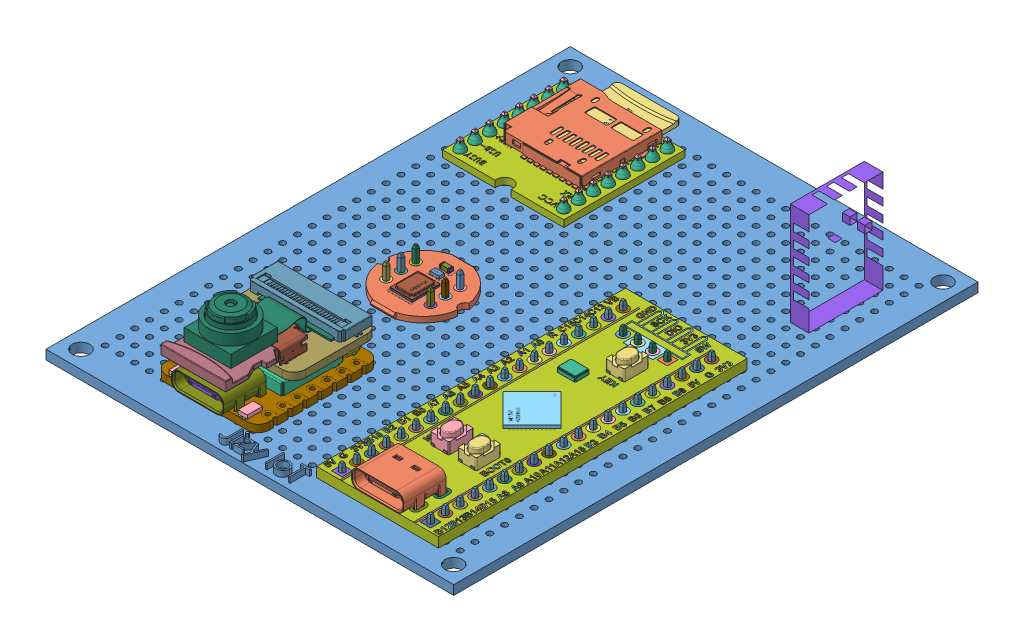
SolidWorks assembly 3D_Final, configuration Default. Lengths in mm.
Overall size (70 33.4 90).
323 component instances, 242 part files, 16 mates.
Components (placement in the parent):
- BoardDong7x9-1: BoardDong7x9 [Default] at (35 1.6 45) x (0 0 -1) z (0 1 0) size (90 70 2.6)
- blackpill v2.0 swi.STEP-1: blackpill v2.0 swi.STEP [Default] at (52.8 1.6 59.37) x (0 0 -1) z (0 1 0) size (53 20.9 10.45)
  - blackpill v2.0.step.STEP-1: blackpill v2.0.step.STEP [Default] at origin size (53 20.9 4.92)
    - USB Type C Port (SMD Type).step.STEP-1: USB Type C Port (SMD Type).step.STEP [Default] at (-19.2 0 3.305) x (0 -1 0) z (0 0 -1) size (8.94 7.9 4.2)
    - PTS810 SJK 250 SMTR LFS--3DModel-STEP-1.step.STEP-1: PTS810 SJK 250 SMTR LFS--3DModel-STEP-1.step.STEP [Default] at (14.5 -1.8498 1.7) x (1 0 0) z (0 -1 0) size (4.6 2.51 3.2)
    - PTS810 SJK 250 SMTR LFS--3DModel-STEP-1.step.STEP-2: PTS810 SJK 250 SMTR LFS--3DModel-STEP-1.step.STEP [Default] at (-11.4 -2.3498 1.7) x (1 0 0) z (0 -1 0) size (4.6 2.51 3.2)
    - PTS810 SJK 250 SMTR LFS--3DModel-STEP-1 v2(Mirror).step.STEP-1: PTS810 SJK 250 SMTR LFS--3DModel-STEP-1 v2(Mirror).step.STEP [Default] at (-11.4 2.3498 1.7) x (1 0 0) z (0 -1 0) size (4.6 2.51 3.2)
    - STM32F411CEU6.step.STEP-1: STM32F411CEU6.step.STEP [Default] at (0 0 1.7) x (-0.707107 -0.707107 0) z (-0.707107 0.707107 0) size (7 0.6 7)
    - ECS-135.60-12-33Q-JES-TR.step.STEP-1: ECS-135.60-12-33Q-JES-TR.step.STEP [Default] at (9.3867 2.3215 1.7) x (0 -1 0) z (-1 0 0) size (3.2 0.8 2.5)
    - DIY_black_pill.step.STEP-1: DIY_black_pill.step.STEP [Default] at origin size (53 20.9 1.7)
    - DIY_black_pill-0.step.STEP-1: DIY_black_pill-0.step.STEP [Default] at origin size (1.8 1.8 1.72)
    - DIY_black_pill-1.step.STEP-1: DIY_black_pill-1.step.STEP [Default] at origin size (1.8 1.8 1.72)
    - DIY_black_pill-2.step.STEP-1: DIY_black_pill-2.step.STEP [Default] at origin size (1.8 1.8 1.72)
    - DIY_black_pill-3.step.STEP-1: DIY_black_pill-3.step.STEP [Default] at origin size (1.8 1.8 1.72)
    - DIY_black_pill-4.step.STEP-1: DIY_black_pill-4.step.STEP [Default] at origin size (1.8 1.8 1.72)
    - DIY_black_pill-5.step.STEP-1: DIY_black_pill-5.step.STEP [Default] at origin size (1.8 1.8 1.72)
    - DIY_black_pill-6.step.STEP-1: DIY_black_pill-6.step.STEP [Default] at origin size (1.8 1.8 1.72)
    - DIY_black_pill-7.step.STEP-1: DIY_black_pill-7.step.STEP [Default] at origin size (1.8 1.8 1.72)
    - DIY_black_pill-8.step.STEP-1: DIY_black_pill-8.step.STEP [Default] at origin size (1.8 1.8 1.72)
    - DIY_black_pill-9.step.STEP-1: DIY_black_pill-9.step.STEP [Default] at origin size (1.8 1.8 1.72)
    - DIY_black_pill-10.step.STEP-1: DIY_black_pill-10.step.STEP [Default] at origin size (1.8 1.8 1.72)
    - DIY_black_pill-11.step.STEP-1: DIY_black_pill-11.step.STEP [Default] at origin size (1.8 1.8 1.72)
    - DIY_black_pill-12.step.STEP-1: DIY_black_pill-12.step.STEP [Default] at origin size (1.8 1.8 1.72)
    - DIY_black_pill-13.step.STEP-1: DIY_black_pill-13.step.STEP [Default] at origin size (1.8 1.8 1.72)
    - DIY_black_pill-14.step.STEP-1: DIY_black_pill-14.step.STEP [Default] at origin size (1.8 1.8 1.72)
    - DIY_black_pill-15.step.STEP-1: DIY_black_pill-15.step.STEP [Default] at origin size (1.8 1.8 1.72)
    - DIY_black_pill-16.step.STEP-1: DIY_black_pill-16.step.STEP [Default] at origin size (1.8 1.8 1.72)
    - DIY_black_pill-17.step.STEP-1: DIY_black_pill-17.step.STEP [Default] at origin size (1.8 1.8 1.72)
    - DIY_black_pill-18.step.STEP-1: DIY_black_pill-18.step.STEP [Default] at origin size (1.8 1.8 1.72)
    - DIY_black_pill-19.step.STEP-1: DIY_black_pill-19.step.STEP [Default] at origin size (1.8 1.8 1.72)
    - DIY_black_pill-20.step.STEP-1: DIY_black_pill-20.step.STEP [Default] at origin size (1.8 1.8 1.72)
    - DIY_black_pill-21.step.STEP-1: DIY_black_pill-21.step.STEP [Default] at origin size (1.8 1.8 1.72)
    - DIY_black_pill-22.step.STEP-1: DIY_black_pill-22.step.STEP [Default] at origin size (1.8 1.8 1.72)
    - DIY_black_pill-23.step.STEP-1: DIY_black_pill-23.step.STEP [Default] at origin size (1.8 1.8 1.72)
    - DIY_black_pill-24.step.STEP-1: DIY_black_pill-24.step.STEP [Default] at origin size (1.8 1.8 1.72)
    - DIY_black_pill-25.step.STEP-1: DIY_black_pill-25.step.STEP [Default] at origin size (1.8 1.8 1.72)
    - DIY_black_pill-26.step.STEP-1: DIY_black_pill-26.step.STEP [Default] at origin size (1.8 1.8 1.72)
    - DIY_black_pill-27.step.STEP-1: DIY_black_pill-27.step.STEP [Default] at origin size (1.8 1.8 1.72)
    - DIY_black_pill-28.step.STEP-1: DIY_black_pill-28.step.STEP [Default] at origin size (1.8 1.8 1.72)
    - DIY_black_pill-29.step.STEP-1: DIY_black_pill-29.step.STEP [Default] at origin size (1.8 1.8 1.72)
    - DIY_black_pill-30.step.STEP-1: DIY_black_pill-30.step.STEP [Default] at origin size (1.8 1.8 1.72)
    - DIY_black_pill-31.step.STEP-1: DIY_black_pill-31.step.STEP [Default] at origin size (1.8 1.8 1.72)
    - DIY_black_pill-32.step.STEP-1: DIY_black_pill-32.step.STEP [Default] at origin size (1.8 1.8 1.72)
    - DIY_black_pill-33.step.STEP-1: DIY_black_pill-33.step.STEP [Default] at origin size (1.8 1.8 1.72)
    - DIY_black_pill-34.step.STEP-1: DIY_black_pill-34.step.STEP [Default] at origin size (1.8 1.8 1.72)
    - DIY_black_pill-35.step.STEP-1: DIY_black_pill-35.step.STEP [Default] at origin size (1.8 1.8 1.72)
    - DIY_black_pill-36.step.STEP-1: DIY_black_pill-36.step.STEP [Default] at origin size (1.8 1.8 1.72)
    - DIY_black_pill-37.step.STEP-1: DIY_black_pill-37.step.STEP [Default] at origin size (1.8 1.8 1.72)
    - DIY_black_pill-38.step.STEP-1: DIY_black_pill-38.step.STEP [Default] at origin size (1.8 1.8 1.72)
    - DIY_black_pill-39.step.STEP-1: DIY_black_pill-39.step.STEP [Default] at origin size (1.8 1.8 1.72)
    - DIY_black_pill-40.step.STEP-1: DIY_black_pill-40.step.STEP [Default] at origin size (51.2 0.3 0.01)
    - DIY_black_pill-41.step.STEP-1: DIY_black_pill-41.step.STEP [Default] at origin size (51.2 0.3 0.01)
    - DIY_black_pill-42.step.STEP-1: DIY_black_pill-42.step.STEP [Default] at origin size (0.93 1 0.01)
    - DIY_black_pill-43.step.STEP-1: DIY_black_pill-43.step.STEP [Default] at origin size (0.94 1.03 0.01)
    - DIY_black_pill-44.step.STEP-1: DIY_black_pill-44.step.STEP [Default] at origin size (0.93 1 0.01)
    - DIY_black_pill-45.step.STEP-1: DIY_black_pill-45.step.STEP [Default] at origin size (0.67 1.02 0.01)
    - DIY_black_pill-46.step.STEP-1: DIY_black_pill-46.step.STEP [Default] at origin size (0.66 1.02 0.01)
    - DIY_black_pill-47.step.STEP-1: DIY_black_pill-47.step.STEP [Default] at origin size (0.84 1 0.01)
    - DIY_black_pill-48.step.STEP-1: DIY_black_pill-48.step.STEP [Default] at origin size (0.67 1.02 0.01)
    - DIY_black_pill-49.step.STEP-1: DIY_black_pill-49.step.STEP [Default] at origin size (0.84 1.01 0.01)
    - DIY_black_pill-50.step.STEP-1: DIY_black_pill-50.step.STEP [Default] at origin size (0.72 1.01 0.01)
    - DIY_black_pill-51.step.STEP-1: DIY_black_pill-51.step.STEP [Default] at origin size (0.84 1 0.01)
    - DIY_black_pill-52.step.STEP-1: DIY_black_pill-52.step.STEP [Default] at origin size (0.67 1 0.01)
    - DIY_black_pill-53.step.STEP-1: DIY_black_pill-53.step.STEP [Default] at origin size (1 1 0.01)
    - DIY_black_pill-54.step.STEP-1: DIY_black_pill-54.step.STEP [Default] at origin size (0.44 1 0.01)
    - DIY_black_pill-55.step.STEP-1: DIY_black_pill-55.step.STEP [Default] at origin size (0.44 1 0.01)
    - DIY_black_pill-56.step.STEP-1: DIY_black_pill-56.step.STEP [Default] at origin size (1 1 0.01)
    - DIY_black_pill-57.step.STEP-1: DIY_black_pill-57.step.STEP [Default] at origin size (0.44 1 0.01)
    - DIY_black_pill-58.step.STEP-1: DIY_black_pill-58.step.STEP [Default] at origin size (0.67 1.02 0.01)
    - DIY_black_pill-59.step.STEP-1: DIY_black_pill-59.step.STEP [Default] at origin size (0.66 1.02 0.01)
    - DIY_black_pill-60.step.STEP-1: DIY_black_pill-60.step.STEP [Default] at origin size (0.67 1 0.01)
    - DIY_black_pill-61.step.STEP-1: DIY_black_pill-61.step.STEP [Default] at origin size (0.84 1 0.01)
    - DIY_black_pill-62.step.STEP-1: DIY_black_pill-62.step.STEP [Default] at origin size (0.44 1 0.01)
    - DIY_black_pill-63.step.STEP-1: DIY_black_pill-63.step.STEP [Default] at origin size (0.66 1.02 0.01)
    - DIY_black_pill-64.step.STEP-1: DIY_black_pill-64.step.STEP [Default] at origin size (0.44 1 0.01)
    - DIY_black_pill-65.step.STEP-1: DIY_black_pill-65.step.STEP [Default] at origin size (0.84 1 0.01)
    - DIY_black_pill-66.step.STEP-1: DIY_black_pill-66.step.STEP [Default] at origin size (0.72 1 0.01)
    - DIY_black_pill-67.step.STEP-1: DIY_black_pill-67.step.STEP [Default] at origin size (0.44 1 0.01)
    - DIY_black_pill-68.step.STEP-1: DIY_black_pill-68.step.STEP [Default] at origin size (0.84 1 0.01)
    - DIY_black_pill-69.step.STEP-1: DIY_black_pill-69.step.STEP [Default] at origin size (1 1 0.01)
    - DIY_black_pill-70.step.STEP-1: DIY_black_pill-70.step.STEP [Default] at origin size (1 1 0.01)
    - DIY_black_pill-71.step.STEP-1: DIY_black_pill-71.step.STEP [Default] at origin size (0.65 1.02 0.01)
    - DIY_black_pill-72.step.STEP-1: DIY_black_pill-72.step.STEP [Default] at origin size (0.44 1 0.01)
    - DIY_black_pill-73.step.STEP-1: DIY_black_pill-73.step.STEP [Default] at origin size (1 1 0.01)
    - DIY_black_pill-74.step.STEP-1: DIY_black_pill-74.step.STEP [Default] at origin size (0.67 1 0.01)
    - DIY_black_pill-75.step.STEP-1: DIY_black_pill-75.step.STEP [Default] at origin size (0.44 1 0.01)
    - DIY_black_pill-76.step.STEP-1: DIY_black_pill-76.step.STEP [Default] at origin size (1 1 0.01)
    - DIY_black_pill-77.step.STEP-1: DIY_black_pill-77.step.STEP [Default] at origin size (0.66 1.02 0.01)
    - DIY_black_pill-78.step.STEP-1: DIY_black_pill-78.step.STEP [Default] at origin size (0.84 1.01 0.01)
    - DIY_black_pill-79.step.STEP-1: DIY_black_pill-79.step.STEP [Default] at origin size (0.67 1.01 0.01)
    - DIY_black_pill-80.step.STEP-1: DIY_black_pill-80.step.STEP [Default] at origin size (0.84 1 0.01)
    - DIY_black_pill-81.step.STEP-1: DIY_black_pill-81.step.STEP [Default] at origin size (0.66 0.99 0.01)
    - DIY_black_pill-82.step.STEP-1: DIY_black_pill-82.step.STEP [Default] at origin size (0.84 1 0.01)
    - DIY_black_pill-83.step.STEP-1: DIY_black_pill-83.step.STEP [Default] at origin size (0.84 1 0.01)
    - DIY_black_pill-84.step.STEP-1: DIY_black_pill-84.step.STEP [Default] at origin size (0.67 1 0.01)
    - DIY_black_pill-85.step.STEP-1: DIY_black_pill-85.step.STEP [Default] at origin size (0.66 1.02 0.01)
    - DIY_black_pill-86.step.STEP-1: DIY_black_pill-86.step.STEP [Default] at origin size (0.66 1.02 0.01)
    - DIY_black_pill-87.step.STEP-1: DIY_black_pill-87.step.STEP [Default] at origin size (0.67 1 0.01)
    - DIY_black_pill-88.step.STEP-1: DIY_black_pill-88.step.STEP [Default] at origin size (0.44 1 0.01)
    - DIY_black_pill-89.step.STEP-1: DIY_black_pill-89.step.STEP [Default] at origin size (0.84 1 0.01)
    - DIY_black_pill-90.step.STEP-1: DIY_black_pill-90.step.STEP [Default] at origin size (1 1 0.01)
    - DIY_black_pill-91.step.STEP-1: DIY_black_pill-91.step.STEP [Default] at origin size (0.84 1 0.01)
    - DIY_black_pill-92.step.STEP-1: DIY_black_pill-92.step.STEP [Default] at origin size (0.44 1 0.01)
    - DIY_black_pill-93.step.STEP-1: DIY_black_pill-93.step.STEP [Default] at origin size (0.87 1.03 0.01)
    - DIY_black_pill-94.step.STEP-1: DIY_black_pill-94.step.STEP [Default] at origin size (0.44 1 0.01)
    - DIY_black_pill-95.step.STEP-1: DIY_black_pill-95.step.STEP [Default] at origin size (0.44 1 0.01)
    - DIY_black_pill-96.step.STEP-1: DIY_black_pill-96.step.STEP [Default] at origin size (0.9 1 0.01)
    - DIY_black_pill-97.step.STEP-1: DIY_black_pill-97.step.STEP [Default] at origin size (0.65 1.02 0.01)
    - DIY_black_pill-98.step.STEP-1: DIY_black_pill-98.step.STEP [Default] at origin size (1 1 0.01)
    - DIY_black_pill-99.step.STEP-1: DIY_black_pill-99.step.STEP [Default] at origin size (0.72 1 0.01)
    - DIY_black_pill-100.step.STEP-1: DIY_black_pill-100.step.STEP [Default] at origin size (1 1 0.01)
    - DIY_black_pill-101.step.STEP-1: DIY_black_pill-101.step.STEP [Default] at origin size (0.67 1.02 0.01)
    - DIY_black_pill-102.step.STEP-1: DIY_black_pill-102.step.STEP [Default] at origin size (0.65 1.02 0.01)
    - DIY_black_pill-103.step.STEP-1: DIY_black_pill-103.step.STEP [Default] at origin size (1 1 0.01)
    - DIY_black_pill-104.step.STEP-1: DIY_black_pill-104.step.STEP [Default] at origin size (0.84 1 0.01)
    - DIY_black_pill-105.step.STEP-1: DIY_black_pill-105.step.STEP [Default] at origin size (0.84 1 0.01)
    - DIY_black_pill-106.step.STEP-1: DIY_black_pill-106.step.STEP [Default] at origin size (0.65 1.02 0.01)
    - DIY_black_pill-107.step.STEP-1: DIY_black_pill-107.step.STEP [Default] at origin size (0.66 1.02 0.01)
    - DIY_black_pill-108.step.STEP-1: DIY_black_pill-108.step.STEP [Default] at origin size (0.66 1.02 0.01)
    - DIY_black_pill-109.step.STEP-1: DIY_black_pill-109.step.STEP [Default] at origin size (0.67 1 0.01)
    - DIY_black_pill-110.step.STEP-1: DIY_black_pill-110.step.STEP [Default] at origin size (0.93 1 0.01)
    - DIY_black_pill-111.step.STEP-1: DIY_black_pill-111.step.STEP [Default] at origin size (0.94 1.03 0.01)
    - DIY_black_pill-112.step.STEP-1: DIY_black_pill-112.step.STEP [Default] at origin size (0.93 1 0.01)
    - DIY_black_pill-113.step.STEP-1: DIY_black_pill-113.step.STEP [Default] at origin size (0.44 1 0.01)
    - DIY_black_pill-114.step.STEP-1: DIY_black_pill-114.step.STEP [Default] at origin size (0.84 1 0.01)
    - DIY_black_pill-115.step.STEP-1: DIY_black_pill-115.step.STEP [Default] at origin size (0.67 1 0.01)
    - DIY_black_pill-116.step.STEP-1: DIY_black_pill-116.step.STEP [Default] at origin size (0.44 1 0.01)
    - DIY_black_pill-117.step.STEP-1: DIY_black_pill-117.step.STEP [Default] at origin size (0.66 0.99 0.01)
    - DIY_black_pill-118.step.STEP-1: DIY_black_pill-118.step.STEP [Default] at origin size (0.84 1 0.01)
    - DIY_black_pill-119.step.STEP-1: DIY_black_pill-119.step.STEP [Default] at origin size (1 1 0.01)
    - DIY_black_pill-120.step.STEP-1: DIY_black_pill-120.step.STEP [Default] at origin size (0.67 1 0.01)
    - DIY_black_pill-121.step.STEP-1: DIY_black_pill-121.step.STEP [Default] at origin size (1 1 0.01)
    - DIY_black_pill-122.step.STEP-1: DIY_black_pill-122.step.STEP [Default] at origin size (0.66 1.02 0.01)
    - DIY_black_pill-123.step.STEP-1: DIY_black_pill-123.step.STEP [Default] at origin size (1 1 0.01)
    - DIY_black_pill-124.step.STEP-1: DIY_black_pill-124.step.STEP [Default] at origin size (0.67 1 0.01)
    - DIY_black_pill-125.step.STEP-1: DIY_black_pill-125.step.STEP [Default] at origin size (0.87 1.03 0.01)
    - DIY_black_pill-126.step.STEP-1: DIY_black_pill-126.step.STEP [Default] at origin size (0.72 1 0.01)
    - DIY_black_pill-127.step.STEP-1: DIY_black_pill-127.step.STEP [Default] at origin size (0.66 1.02 0.01)
    - DIY_black_pill-128.step.STEP-1: DIY_black_pill-128.step.STEP [Default] at origin size (0.87 1.03 0.01)
    - DIY_black_pill-129.step.STEP-1: DIY_black_pill-129.step.STEP [Default] at origin size (0.93 1 0.01)
    - DIY_black_pill-130.step.STEP-1: DIY_black_pill-130.step.STEP [Default] at origin size (0.44 1 0.01)
    - DIY_black_pill-131.step.STEP-1: DIY_black_pill-131.step.STEP [Default] at origin size (2.55 1.5 1.72)
    - DIY_black_pill-132.step.STEP-1: DIY_black_pill-132.step.STEP [Default] at origin size (2.6 1.5 1.72)
    - DIY_black_pill-133.step.STEP-1: DIY_black_pill-133.step.STEP [Default] at origin size (2.55 1.5 1.72)
    - DIY_black_pill-134.step.STEP-1: DIY_black_pill-134.step.STEP [Default] at origin size (2.6 1.5 1.72)
    - DIY_black_pill-135.step.STEP-1: DIY_black_pill-135.step.STEP [Default] at origin size (1 1 0.01)
    - DIY_black_pill-136.step.STEP-1: DIY_black_pill-136.step.STEP [Default] at origin size (0.67 1.01 0.01)
    - DIY_black_pill-137.step.STEP-1: DIY_black_pill-137.step.STEP [Default] at origin size (1.8 1.8 1.72)
    - DIY_black_pill-138.step.STEP-1: DIY_black_pill-138.step.STEP [Default] at origin size (1.8 1.8 1.72)
    - DIY_black_pill-139.step.STEP-1: DIY_black_pill-139.step.STEP [Default] at origin size (1.8 1.8 1.72)
    - DIY_black_pill-140.step.STEP-1: DIY_black_pill-140.step.STEP [Default] at origin size (1.8 1.8 1.72)
    - DIY_black_pill-141.step.STEP-1: DIY_black_pill-141.step.STEP [Default] at origin size (8.17 10.16 0.01)
    - DIY_black_pill-142.step.STEP-1: DIY_black_pill-142.step.STEP [Default] at origin size (1.31 1 0.01)
    - DIY_black_pill-143.step.STEP-1: DIY_black_pill-143.step.STEP [Default] at origin size (0.93 1 0.01)
    - DIY_black_pill-144.step.STEP-1: DIY_black_pill-144.step.STEP [Default] at origin size (0.84 1 0.01)
    - DIY_black_pill-145.step.STEP-1: DIY_black_pill-145.step.STEP [Default] at origin size (0.2 1 0.01)
    - DIY_black_pill-146.step.STEP-1: DIY_black_pill-146.step.STEP [Default] at origin size (0.87 1.03 0.01)
    - DIY_black_pill-147.step.STEP-1: DIY_black_pill-147.step.STEP [Default] at origin size (0.94 1.03 0.01)
    - DIY_black_pill-148.step.STEP-1: DIY_black_pill-148.step.STEP [Default] at origin size (0.79 1 0.01)
    - DIY_black_pill-149.step.STEP-1: DIY_black_pill-149.step.STEP [Default] at origin size (0.84 1 0.01)
    - DIY_black_pill-150.step.STEP-1: DIY_black_pill-150.step.STEP [Default] at origin size (0.9 1 0.01)
    - DIY_black_pill-151.step.STEP-1: DIY_black_pill-151.step.STEP [Default] at origin size (0.81 1.03 0.01)
    - DIY_black_pill-152.step.STEP-1: DIY_black_pill-152.step.STEP [Default] at origin size (0.97 1.03 0.01)
    - DIY_black_pill-153.step.STEP-1: DIY_black_pill-153.step.STEP [Default] at origin size (0.66 1.02 0.01)
    - DIY_black_pill-154.step.STEP-1: DIY_black_pill-154.step.STEP [Default] at origin size (0.66 1.02 0.01)
    - DIY_black_pill-155.step.STEP-1: DIY_black_pill-155.step.STEP [Default] at origin size (0.81 1.03 0.01)
    - DIY_black_pill-156.step.STEP-1: DIY_black_pill-156.step.STEP [Default] at origin size (0.9 1 0.01)
    - DIY_black_pill-157.step.STEP-1: DIY_black_pill-157.step.STEP [Default] at origin size (0.81 1.03 0.01)
    - DIY_black_pill-158.step.STEP-1: DIY_black_pill-158.step.STEP [Default] at origin size (0.97 1.03 0.01)
    - DIY_black_pill-159.step.STEP-1: DIY_black_pill-159.step.STEP [Default] at origin size (0.97 1.03 0.01)
    - DIY_black_pill-160.step.STEP-1: DIY_black_pill-160.step.STEP [Default] at origin size (1.01 0.91 0.01)
    - DIY_black_pill-161.step.STEP-1: DIY_black_pill-161.step.STEP [Default] at origin size (1 0.94 0.01)
    - DIY_black_pill-162.step.STEP-1: DIY_black_pill-162.step.STEP [Default] at origin size (1 0.77 0.01)
    - DIY_black_pill-163.step.STEP-1: DIY_black_pill-163.step.STEP [Default] at origin size (0.79 1 0.01)
    - DIY_black_pill-164.step.STEP-1: DIY_black_pill-164.step.STEP [Default] at origin size (0.65 1.02 0.01)
    - DIY_black_pill-165.step.STEP-1: DIY_black_pill-165.step.STEP [Default] at origin size (0.84 1 0.01)
    - DIY_black_pill-166.step.STEP-1: DIY_black_pill-166.step.STEP [Default] at origin size (0.79 1 0.01)
    - DIY_black_pill-167.step.STEP-1: DIY_black_pill-167.step.STEP [Default] at origin size (0.79 1 0.01)
  - 1x20 Male Pin Header.STEP-1: 1x20 Male Pin Header.STEP [Default] at (23.26 -7.6 0) x (-1 0 0) z (0 -1 0) size (50.8 8.54 2.5)
  - 1x20 Male Pin Header.STEP-2: 1x20 Male Pin Header.STEP [Default] at (23.26 7.6 0) x (-1 0 0) z (0 -1 0) size (50.8 8.54 2.5)
  - 1x4 Male Pin Header.STEP-1: 1x4 Male Pin Header.STEP [Default] at (19.45 -3.81 0) x (0 1 0) z (-1 0 0) size (10.17 8.54 2.5)
- Seeed Studio XIAO-ESP32-S3-Sense-1: Seeed Studio XIAO-ESP32-S3-Sense [Default] at (16.1886 1.85 72.4693) x (0 0 1) z (-1 0 0) size (24.36 13.98 17.79)
  - Seeed Studio XIAO-ESP32-S3-Sense.step-1: Seeed Studio XIAO-ESP32-S3-Sense.step [Default] at origin size (24.36 13.98 17.79)
    - Seeed Studio XIAO-ESP32-S3 (Sense).step-1: Seeed Studio XIAO-ESP32-S3 (Sense).step [Default] at origin size (22.49 4.48 17.79)
      - USB TYPE C PORT.step-1: USB TYPE C PORT.step [Default] at (4.3161 13.395 -12.1571) x (0 0 -1) z (0 -1 0) size (8.94 7.9 4.2)
        - USB TYPE C PORT (1).step-1: USB TYPE C PORT (1).step [Default] at (-3.0192 1.0963 5.395) size (8.94 7.9 4.2)
          - BOSS-EXTRUDE14_8_.step-1: BOSS-EXTRUDE14_8_.step [Default] at (-3.0192 1.0963 5.395) size (0.6 1 0.3)
          - BOSS-EXTRUDE7_4_.step-1: BOSS-EXTRUDE7_4_.step [Default] at (-3.0192 1.0963 5.395) size (0.3 3.78 0.75)
          - BOSS-EXTRUDE7_3_.step-1: BOSS-EXTRUDE7_3_.step [Default] at (-3.0192 1.0963 5.395) size (0.3 3.78 0.75)
          - BOSS-EXTRUDE14_4_.step-1: BOSS-EXTRUDE14_4_.step [Default] at (-3.0192 1.0963 5.395) size (0.3 1 0.3)
          - BOSS-EXTRUDE14_2_.step-1: BOSS-EXTRUDE14_2_.step [Default] at (-3.0192 1.0963 5.395) size (0.6 1 0.3)
          - BOSS-EXTRUDE14_11_.step-1: BOSS-EXTRUDE14_11_.step [Default] at (-3.0192 1.0963 5.395) size (0.3 1 0.3)
          - BOSS-EXTRUDE7_7_.step-1: BOSS-EXTRUDE7_7_.step [Default] at (-3.0192 1.0963 5.395) size (0.3 3.78 0.75)
          - BOSS-EXTRUDE14_9_.step-1: BOSS-EXTRUDE14_9_.step [Default] at (-3.0192 1.0963 5.395) size (0.3 1 0.3)
          - BOSS-EXTRUDE14_3_.step-1: BOSS-EXTRUDE14_3_.step [Default] at (-3.0192 1.0963 5.395) size (0.3 1 0.3)
          - BOSS-EXTRUDE14_7_.step-1: BOSS-EXTRUDE14_7_.step [Default] at (-3.0192 1.0963 5.395) size (0.6 1 0.3)
          - MIRROR2.step-1: MIRROR2.step [Default] at (-3.0192 1.0963 5.395) size (6.7 4.6 0.7)
          - BOSS-EXTRUDE14_5_.step-1: BOSS-EXTRUDE14_5_.step [Default] at (-3.0192 1.0963 5.395) size (0.3 1 0.3)
          - BOSS-EXTRUDE14_12_.step-1: BOSS-EXTRUDE14_12_.step [Default] at (-3.0192 1.0963 5.395) size (0.3 1 0.3)
          - BOSS-EXTRUDE7_8_.step-1: BOSS-EXTRUDE7_8_.step [Default] at (-3.0192 1.0963 5.395) size (0.3 3.78 0.75)
          - BOSS-EXTRUDE7_1_.step-1: BOSS-EXTRUDE7_1_.step [Default] at (-3.0192 1.0963 5.395) size (0.3 3.78 0.75)
          - BOSS-EXTRUDE14_10_.step-1: BOSS-EXTRUDE14_10_.step [Default] at (-3.0192 1.0963 5.395) size (0.3 1 0.3)
          - BOSS-EXTRUDE7_9_.step-1: BOSS-EXTRUDE7_9_.step [Default] at (-3.0192 1.0963 5.395) size (0.3 3.78 0.75)
          - BOSS-EXTRUDE14_6_.step-1: BOSS-EXTRUDE14_6_.step [Default] at (-3.0192 1.0963 5.395) size (0.6 1 0.3)
          - CHAMFER9.step-1: CHAMFER9.step [Default] at (-3.0192 1.0963 5.395) size (8.94 7.3 4.2)
          - BOSS-EXTRUDE14_1_.step-1: BOSS-EXTRUDE14_1_.step [Default] at (-3.0192 1.0963 5.395) size (0.3 1 0.3)
          - BOSS-EXTRUDE7_6_.step-1: BOSS-EXTRUDE7_6_.step [Default] at (-3.0192 1.0963 5.395) size (0.3 3.78 0.75)
          - BOSS-EXTRUDE7_2_.step-1: BOSS-EXTRUDE7_2_.step [Default] at (-3.0192 1.0963 5.395) size (0.3 3.78 0.75)
          - CUT-EXTRUDE5.step-1: CUT-EXTRUDE5.step [Default] at (-3.0192 1.0963 5.395) size (8.54 2 3.59)
          - BOSS-EXTRUDE7_5_.step-1: BOSS-EXTRUDE7_5_.step [Default] at (-3.0192 1.0963 5.395) size (0.3 3.78 0.75)
      - SKTAAAE010 v1.step-1: SKTAAAE010 v1.step [Default] at (10.7092 1 -12.0449) x (1 0 0) z (0 1 0) size (3.09 1.6 0.73)
        - Body.step-1: Body.step [Default] at (0 0 0.1) size (2.6 1.6 0.63)
        - Pins.step-1: Pins.step [Default] at origin size (3.09 1.19 0.1)
      - SKTAAAE010 v1.step-2: SKTAAAE010 v1.step [Default] at (10.6911 1 -0.1868) x (1 0 0) z (0 1 0) size (3.09 1.6 0.73)
        - Body.step-1: Body.step [Default] at (0 0 0.1) size (2.6 1.6 0.63)
        - Pins.step-1: Pins.step [Default] at origin size (3.09 1.19 0.1)
      - Shield.step-1: Shield.step [Default] at origin size (10.6 2.7 12.6)
      - U.FL-R-SMT-1_10_ v1.step-1: U.FL-R-SMT-1_10_ v1.step [Default] at (-6.9517 1 -10.8381) x (1 0 0) z (0 1 0) size (3 3.1 1.25)
      - DF40C-30DP-0.4V_51_ v1.step-1: DF40C-30DP-0.4V_51_ v1.step [Default] at (-6.0667 1.65 -7.7227) size (2.97 1.14 7.52)
      - Seeed Studio XIAO-ESP32-S3 (Sense)-0.step-1: Seeed Studio XIAO-ESP32-S3 (Sense)-0.step [Default] at origin size (20.97 1.28 17.79)
    - Sense Expansion Board.step-1: Sense Expansion Board.step [Default] at (-0.3 4.5 0) x (-1 0 0) z (0 0 1) size (24.36 7.23 16.78)
      - DF40HC(3.0)-30DS.step-1: DF40HC(3.0)-30DS.step [Default] at (6.4217 1.57 -3.0777) x (-1 0 0) z (0 0 1) size (3.38 2.9 8.6)
      - 10067099-200LF v1.step-1: 10067099-200LF v1.step [Default] at (-1.3077 -2.08 -6.0846) x (0 0 -1) z (-1 0 0) size (11.4 2.65 5.5)
      - PCB.step-1: PCB.step [Default] at origin size (14.68 1.25 16.78)
      - MicroSD v2.step-1: MicroSD v2.step [Default] at (-8.16 -2.1 -6.9267) x (1 0 0) z (0 0 -1) size (15.06 1.66 11.19)
      - JUSHUO AFC01-S24FCA-00.step-1: JUSHUO AFC01-S24FCA-00.step [Default] at (6.9932 -0.67 -6.0797) x (0 0 1) z (0 -1 0) size (16.2 6.01 2.01)
    - Camer Module.step-1: Camer Module.step [Default] at (-7.2 6 -13) size (19.95 8.11 12.5)
- INMP441 I2S Microphone Module v15-1: INMP441 I2S Microphone Module v15 [Default] at (23.57 1.6 48.81) size (13.77 11.25 14.24)
  - INMP441 I2S Microphone Module v15.step-1: INMP441 I2S Microphone Module v15.step [Default] at origin size (13.77 11.25 14.24)
    - C0603_070.step-1: C0603_070.step [Default] at (0 8.5 0) x (1 0 0) z (0 1 0) size (1.6 0.8 0.7)
      - C0603_070_1.step-1: C0603_070_1.step [Default] at origin size (1.6 0.8 0.7)
        - Part 3.step-1: Part 3.step [Default] at (0 4 -7.535) size (1.4 0.77 0.67)
        - Part 2.step-1: Part 2.step [Default] at (0 4 -7.535) size (0.2 0.8 0.7)
        - Part 1.step-1: Part 1.step [Default] at (0 4 -7.535) size (0.2 0.8 0.7)
    - 0603 Resistor.step-1: 0603 Resistor.step [Default] at (0 0.98 -2.4) x (1 0 0) z (0 1 0) size (1.6 0.9 0.5)
    - INMP441 I2S Microphone Module.step-1: INMP441 I2S Microphone Module.step [Default] at origin size (13.77 1 14.24)
    - INMP441 I2S Microphone Module-0.step-1: INMP441 I2S Microphone Module-0.step [Default] at origin size (1.6 1 1.6)
    - INMP441 I2S Microphone Module-1.step-1: INMP441 I2S Microphone Module-1.step [Default] at origin size (1.6 1 1.6)
    - INMP441 I2S Microphone Module-2.step-1: INMP441 I2S Microphone Module-2.step [Default] at origin size (1.6 1 1.6)
    - INMP441 I2S Microphone Module-3.step-1: INMP441 I2S Microphone Module-3.step [Default] at origin size (1.6 1 1.6)
    - INMP441 I2S Microphone Module-4.step-1: INMP441 I2S Microphone Module-4.step [Default] at origin size (1.6 1 1.6)
    - INMP441 I2S Microphone Module-5.step-1: INMP441 I2S Microphone Module-5.step [Default] at origin size (1.6 1 1.6)
    - INMP441 I2S Microphone Module-6.step-1: INMP441 I2S Microphone Module-6.step [Default] at origin size (1.6 1 1.6)
    - INMP441 I2S Microphone Module-7.step-1: INMP441 I2S Microphone Module-7.step [Default] at origin size (3.79 0.3 4.79)
    - INMP441 I2S Microphone Module-8.step-1: INMP441 I2S Microphone Module-8.step [Default] at origin size (3.79 0.41 4.79)
    - INMP441 I2S Microphone Module-9.step-1: INMP441 I2S Microphone Module-9.step [Default] at origin size (0.65 11.25 0.65)
    - INMP441 I2S Microphone Module-10.step-1: INMP441 I2S Microphone Module-10.step [Default] at origin size (2.55 2.5 7.63)
    - INMP441 I2S Microphone Module-11.step-1: INMP441 I2S Microphone Module-11.step [Default] at origin size (0.65 11.25 0.65)
    - INMP441 I2S Microphone Module-12.step-1: INMP441 I2S Microphone Module-12.step [Default] at origin size (0.65 11.25 0.65)
    - INMP441 I2S Microphone Module-13.step-1: INMP441 I2S Microphone Module-13.step [Default] at origin size (0.65 11.25 0.65)
    - INMP441 I2S Microphone Module-14.step-1: INMP441 I2S Microphone Module-14.step [Default] at origin size (2.55 2.5 7.63)
    - INMP441 I2S Microphone Module-15.step-1: INMP441 I2S Microphone Module-15.step [Default] at origin size (0.65 11.25 0.65)
    - INMP441 I2S Microphone Module-16.step-1: INMP441 I2S Microphone Module-16.step [Default] at origin size (0.65 11.25 0.65)
- DFPlayer Mini Assem v1.step-1: DFPlayer Mini Assem v1.step [Default] at (15.95 1.6 17.06) x (-1 0 0) z (0 0 -1) size (20.8 11.2 23.46)
  - SD card Assem^DFPlayer Mini Assem v1.step-1: SD card Assem^DFPlayer Mini Assem v1.step [Default] at (-198.0203 122.5536 -43.8714) x (0 1 0) z (1 0 0) size (2.44 17.9 16) (virtual)
    - CD card slot^SD card Assem_DFPlayer Mini Assem v1.step-1: CD card slot^SD card Assem_DFPlayer Mini Assem v1.step [Default] at (-120.5536 47.0914 197.6703) x (0 0 1) z (1 0 0) size (16 15 2.44) (virtual)
    - Micro sd card^SD card Assem_DFPlayer Mini Assem v1.step-1: Micro sd card^SD card Assem_DFPlayer Mini Assem v1.step [Default] at (-120.5536 45.5089 151.9853) x (0 0 1) z (1 0 0) size (11 15 0.95) (virtual)
  - DFPlayer Mini Pin.step-1: DFPlayer Mini Pin.step [Default] at (8.89 0 8.89) x (0 0 -1) z (0 -1 0) size (2.54 2.54 11.2)
    - 11_20mm pin.step-1: 11_20mm pin.step [Default] at (0 0 2.6) size (0.63 0.63 11.2)
    - Pin Header 1x12 TH Pitch 2.step-1: Pin Header 1x12 TH Pitch 2.step [Default] at (-27.94 0 -0.0014) size (2.54 2.54 2.8)
    - solder.step-1: solder.step [Default] at (0 0 -1.15) x (1 0 0) z (0 1 0) size (1.8 1.45 1.8)
  - DFPlayer Mini Pin.step-2: DFPlayer Mini Pin.step [Default] at (-8.89 0 8.89) x (0 0 1) z (0 -1 0) size (2.54 2.54 11.2)
    - 11_20mm pin.step-1: 11_20mm pin.step [Default] at (0 0 2.6) size (0.63 0.63 11.2)
    - Pin Header 1x12 TH Pitch 2.step-1: Pin Header 1x12 TH Pitch 2.step [Default] at (-27.94 0 -0.0014) size (2.54 2.54 2.8)
    - solder.step-1: solder.step [Default] at (0 0 -1.15) x (1 0 0) z (0 1 0) size (1.8 1.45 1.8)
  - DFPlayer Mini Pin.step-3: DFPlayer Mini Pin.step [Default] at (-8.89 0 6.35) x (0 0 1) z (0 -1 0) size (2.54 2.54 11.2)
    - 11_20mm pin.step-1: 11_20mm pin.step [Default] at (0 0 2.6) size (0.63 0.63 11.2)
    - Pin Header 1x12 TH Pitch 2.step-1: Pin Header 1x12 TH Pitch 2.step [Default] at (-27.94 0 -0.0014) size (2.54 2.54 2.8)
    - solder.step-1: solder.step [Default] at (0 0 -1.15) x (1 0 0) z (0 1 0) size (1.8 1.45 1.8)
  - DFPlayer Mini Pin.step-4: DFPlayer Mini Pin.step [Default] at (-8.89 0 3.81) x (0 0 1) z (0 -1 0) size (2.54 2.54 11.2)
    - 11_20mm pin.step-1: 11_20mm pin.step [Default] at (0 0 2.6) size (0.63 0.63 11.2)
    - Pin Header 1x12 TH Pitch 2.step-1: Pin Header 1x12 TH Pitch 2.step [Default] at (-27.94 0 -0.0014) size (2.54 2.54 2.8)
    - solder.step-1: solder.step [Default] at (0 0 -1.15) x (1 0 0) z (0 1 0) size (1.8 1.45 1.8)
  - DFPlayer Mini Pin.step-5: DFPlayer Mini Pin.step [Default] at (-8.89 0 1.27) x (0 0 1) z (0 -1 0) size (2.54 2.54 11.2)
    - 11_20mm pin.step-1: 11_20mm pin.step [Default] at (0 0 2.6) size (0.63 0.63 11.2)
    - Pin Header 1x12 TH Pitch 2.step-1: Pin Header 1x12 TH Pitch 2.step [Default] at (-27.94 0 -0.0014) size (2.54 2.54 2.8)
    - solder.step-1: solder.step [Default] at (0 0 -1.15) x (1 0 0) z (0 1 0) size (1.8 1.45 1.8)
  - DFPlayer Mini Pin.step-6: DFPlayer Mini Pin.step [Default] at (-8.89 0 -1.27) x (0 0 1) z (0 -1 0) size (2.54 2.54 11.2)
    - 11_20mm pin.step-1: 11_20mm pin.step [Default] at (0 0 2.6) size (0.63 0.63 11.2)
    - Pin Header 1x12 TH Pitch 2.step-1: Pin Header 1x12 TH Pitch 2.step [Default] at (-27.94 0 -0.0014) size (2.54 2.54 2.8)
    - solder.step-1: solder.step [Default] at (0 0 -1.15) x (1 0 0) z (0 1 0) size (1.8 1.45 1.8)
  - DFPlayer Mini Pin.step-7: DFPlayer Mini Pin.step [Default] at (-8.89 0 -3.81) x (0 0 1) z (0 -1 0) size (2.54 2.54 11.2)
    - 11_20mm pin.step-1: 11_20mm pin.step [Default] at (0 0 2.6) size (0.63 0.63 11.2)
    - Pin Header 1x12 TH Pitch 2.step-1: Pin Header 1x12 TH Pitch 2.step [Default] at (-27.94 0 -0.0014) size (2.54 2.54 2.8)
    - solder.step-1: solder.step [Default] at (0 0 -1.15) x (1 0 0) z (0 1 0) size (1.8 1.45 1.8)
  - DFPlayer Mini Pin.step-8: DFPlayer Mini Pin.step [Default] at (-8.89 0 -6.35) x (0 0 1) z (0 -1 0) size (2.54 2.54 11.2)
    - 11_20mm pin.step-1: 11_20mm pin.step [Default] at (0 0 2.6) size (0.63 0.63 11.2)
    - Pin Header 1x12 TH Pitch 2.step-1: Pin Header 1x12 TH Pitch 2.step [Default] at (-27.94 0 -0.0014) size (2.54 2.54 2.8)
    - solder.step-1: solder.step [Default] at (0 0 -1.15) x (1 0 0) z (0 1 0) size (1.8 1.45 1.8)
  - DFPlayer Mini Pin.step-9: DFPlayer Mini Pin.step [Default] at (-8.89 0 -8.89) x (0 0 1) z (0 -1 0) size (2.54 2.54 11.2)
    - 11_20mm pin.step-1: 11_20mm pin.step [Default] at (0 0 2.6) size (0.63 0.63 11.2)
    - Pin Header 1x12 TH Pitch 2.step-1: Pin Header 1x12 TH Pitch 2.step [Default] at (-27.94 0 -0.0014) size (2.54 2.54 2.8)
    - solder.step-1: solder.step [Default] at (0 0 -1.15) x (1 0 0) z (0 1 0) size (1.8 1.45 1.8)
  - DFPlayer Mini Pin.step-10: DFPlayer Mini Pin.step [Default] at (8.89 0 6.35) x (0 0 -1) z (0 -1 0) size (2.54 2.54 11.2)
    - 11_20mm pin.step-1: 11_20mm pin.step [Default] at (0 0 2.6) size (0.63 0.63 11.2)
    - Pin Header 1x12 TH Pitch 2.step-1: Pin Header 1x12 TH Pitch 2.step [Default] at (-27.94 0 -0.0014) size (2.54 2.54 2.8)
    - solder.step-1: solder.step [Default] at (0 0 -1.15) x (1 0 0) z (0 1 0) size (1.8 1.45 1.8)
  - DFPlayer Mini Pin.step-11: DFPlayer Mini Pin.step [Default] at (8.89 0 3.81) x (0 0 -1) z (0 -1 0) size (2.54 2.54 11.2)
    - 11_20mm pin.step-1: 11_20mm pin.step [Default] at (0 0 2.6) size (0.63 0.63 11.2)
    - Pin Header 1x12 TH Pitch 2.step-1: Pin Header 1x12 TH Pitch 2.step [Default] at (-27.94 0 -0.0014) size (2.54 2.54 2.8)
    - solder.step-1: solder.step [Default] at (0 0 -1.15) x (1 0 0) z (0 1 0) size (1.8 1.45 1.8)
  - DFPlayer Mini Pin.step-12: DFPlayer Mini Pin.step [Default] at (8.89 0 1.27) x (0 0 -1) z (0 -1 0) size (2.54 2.54 11.2)
    - 11_20mm pin.step-1: 11_20mm pin.step [Default] at (0 0 2.6) size (0.63 0.63 11.2)
    - Pin Header 1x12 TH Pitch 2.step-1: Pin Header 1x12 TH Pitch 2.step [Default] at (-27.94 0 -0.0014) size (2.54 2.54 2.8)
    - solder.step-1: solder.step [Default] at (0 0 -1.15) x (1 0 0) z (0 1 0) size (1.8 1.45 1.8)
  - DFPlayer Mini Pin.step-13: DFPlayer Mini Pin.step [Default] at (8.89 0 -1.27) x (0 0 -1) z (0 -1 0) size (2.54 2.54 11.2)
    - 11_20mm pin.step-1: 11_20mm pin.step [Default] at (0 0 2.6) size (0.63 0.63 11.2)
    - Pin Header 1x12 TH Pitch 2.step-1: Pin Header 1x12 TH Pitch 2.step [Default] at (-27.94 0 -0.0014) size (2.54 2.54 2.8)
    - solder.step-1: solder.step [Default] at (0 0 -1.15) x (1 0 0) z (0 1 0) size (1.8 1.45 1.8)
  - DFPlayer Mini Pin.step-14: DFPlayer Mini Pin.step [Default] at (8.89 0 -3.81) x (0 0 -1) z (0 -1 0) size (2.54 2.54 11.2)
    - 11_20mm pin.step-1: 11_20mm pin.step [Default] at (0 0 2.6) size (0.63 0.63 11.2)
    - Pin Header 1x12 TH Pitch 2.step-1: Pin Header 1x12 TH Pitch 2.step [Default] at (-27.94 0 -0.0014) size (2.54 2.54 2.8)
    - solder.step-1: solder.step [Default] at (0 0 -1.15) x (1 0 0) z (0 1 0) size (1.8 1.45 1.8)
  - DFPlayer Mini Pin.step-15: DFPlayer Mini Pin.step [Default] at (8.89 0 -6.35) x (0 0 -1) z (0 -1 0) size (2.54 2.54 11.2)
    - 11_20mm pin.step-1: 11_20mm pin.step [Default] at (0 0 2.6) size (0.63 0.63 11.2)
    - Pin Header 1x12 TH Pitch 2.step-1: Pin Header 1x12 TH Pitch 2.step [Default] at (-27.94 0 -0.0014) size (2.54 2.54 2.8)
    - solder.step-1: solder.step [Default] at (0 0 -1.15) x (1 0 0) z (0 1 0) size (1.8 1.45 1.8)
  - DFPlayer Mini Pin.step-16: DFPlayer Mini Pin.step [Default] at (8.89 0 -8.89) x (0 0 -1) z (0 -1 0) size (2.54 2.54 11.2)
    - 11_20mm pin.step-1: 11_20mm pin.step [Default] at (0 0 2.6) size (0.63 0.63 11.2)
    - Pin Header 1x12 TH Pitch 2.step-1: Pin Header 1x12 TH Pitch 2.step [Default] at (-27.94 0 -0.0014) size (2.54 2.54 2.8)
    - solder.step-1: solder.step [Default] at (0 0 -1.15) x (1 0 0) z (0 1 0) size (1.8 1.45 1.8)
  - DFPlayer Mini PCB^DFPlayer Mini Assem v1.step-1: DFPlayer Mini PCB^DFPlayer Mini Assem v1.step [Default] at origin size (20.8 1.15 20.8) (virtual)
- DHT22-1: DHT22 [Default] at (60.4 1.6 20.87) x (0 0 -1) z (0 1 0) size (15.33 7.8 27.74)
Mates (geometry in assembly coordinates):
- Concentric1: concentric aligned: cylinder of BoardDong7x9-1 through (60.4 0 84.37) axis (0 1 0) radius 0.5; circle of blackpill v2.0 swi.STEP-1/blackpill v2.0.step.STEP-1/DIY_black_pill-20.step.STEP-1
- Parallel1: parallel aligned: plane of BoardDong7x9-1 through (70 0 0) normal (1 0 0); plane of blackpill v2.0 swi.STEP-1/blackpill v2.0.step.STEP-1/DIY_black_pill.step.STEP-1 through (63.25 1.6 85.87) normal (1 0 0)
- Coincident2: coincident anti-aligned: plane of BoardDong7x9-1 through (35 1.6 45) normal (0 1 0); plane of blackpill v2.0 swi.STEP-1/blackpill v2.0.step.STEP-1/DIY_black_pill.step.STEP-1 through (52.8 1.6 59.37) normal (0 -1 0)
- Parallel2: parallel aligned: plane of BoardDong7x9-1 through (70 0 90) normal (0 0 1); plane of Seeed Studio XIAO-ESP32-S3-Sense-1/Seeed Studio XIAO-ESP32-S3-Sense.step-1/Seeed Studio XIAO-ESP32-S3 (Sense).step-1/Seeed Studio XIAO-ESP32-S3 (Sense)-0.step-1 through (15.315 1.85 84.751) normal (0 0 1)
- Parallel3: parallel aligned: plane of BoardDong7x9-1 through (0 0 0) normal (-1 0 0); plane of Seeed Studio XIAO-ESP32-S3-Sense-1/Seeed Studio XIAO-ESP32-S3-Sense.step-1/Sense Expansion Board.step-1/PCB.step-1 through (13.91 5.78 62.996) normal (-1 0 0)
- Concentric2: concentric aligned: circle of BoardDong7x9-1; cylinder of Seeed Studio XIAO-ESP32-S3-Sense-1/Seeed Studio XIAO-ESP32-S3-Sense.step-1/Seeed Studio XIAO-ESP32-S3 (Sense).step-1/Seeed Studio XIAO-ESP32-S3 (Sense)-0.step-1 through (29.92 1.85 81.83) axis (0 1 0) radius 0.375
- Coincident5: coincident anti-aligned: plane of BoardDong7x9-1 through (35 1.6 45) normal (0 1 0); plane of Seeed Studio XIAO-ESP32-S3-Sense-1/Seeed Studio XIAO-ESP32-S3-Sense.step-1/Seeed Studio XIAO-ESP32-S3 (Sense).step-1/Seeed Studio XIAO-ESP32-S3 (Sense)-0.step-1 through (22.3 1.6 74.2735) normal (0 -1 0)
- Concentric3: concentric anti-aligned: line of BoardDong7x9-1 through (27.38 0 51.35) axis (0 1 0); circle of INMP441 I2S Microphone Module v15-1/INMP441 I2S Microphone Module v15.step-1/INMP441 I2S Microphone Module-5.step-1
- Parallel4: parallel aligned: plane of blackpill v2.0 swi.STEP-1/blackpill v2.0.step.STEP-1/DIY_black_pill.step.STEP-1 through (63.25 1.6 85.87) normal (1 0 0); plane of INMP441 I2S Microphone Module v15-1/INMP441 I2S Microphone Module v15.step-1/INMP441 I2S Microphone Module-7.step-1 through (25.465 2.58 52.6) normal (1 0 0)
- Coincident7: coincident anti-aligned: plane of BoardDong7x9-1 through (35 1.6 45) normal (0 1 0); plane of INMP441 I2S Microphone Module v15-1/INMP441 I2S Microphone Module v15.step-1/INMP441 I2S Microphone Module.step-1 through (23.57 1.6 48.81) normal (0 -1 0)
- Coincident11: coincident anti-aligned: plane of BoardDong7x9-1 through (35 1.6 45) normal (0 1 0); plane of DHT22-1 through (61.695 1.6 24.71) normal (0 -1 0)
- Parallel7: parallel anti-aligned: plane of BoardDong7x9-1 through (70 0 0) normal (1 0 0); plane of DHT22-1 through (57.895 11.7 17.06) normal (-1 0 0)
- Concentric5: concentric anti-aligned: line of BoardDong7x9-1 through (60.4 0 18.33) axis (0 1 0); circle of DHT22-1
- Concentric7: concentric anti-aligned: line of BoardDong7x9-1 through (7.06 0 8.17) axis (0 1 0); circle of DFPlayer Mini Assem v1.step-1/DFPlayer Mini Pin.step-1/solder.step-1
- Parallel9: parallel aligned: plane of BoardDong7x9-1 through (0 0 0) normal (-1 0 0); plane of DFPlayer Mini Assem v1.step-1/DFPlayer Mini PCB^DFPlayer Mini Assem v1.step-1 through (5.55 2.75 27.46) normal (-1 0 0)
- Coincident17: coincident anti-aligned: plane of BoardDong7x9-1 through (35 1.6 45) normal (0 1 0); plane of DFPlayer Mini Assem v1.step-1/DFPlayer Mini PCB^DFPlayer Mini Assem v1.step-1 through (15.95 1.6 17.06) normal (0 -1 0)
